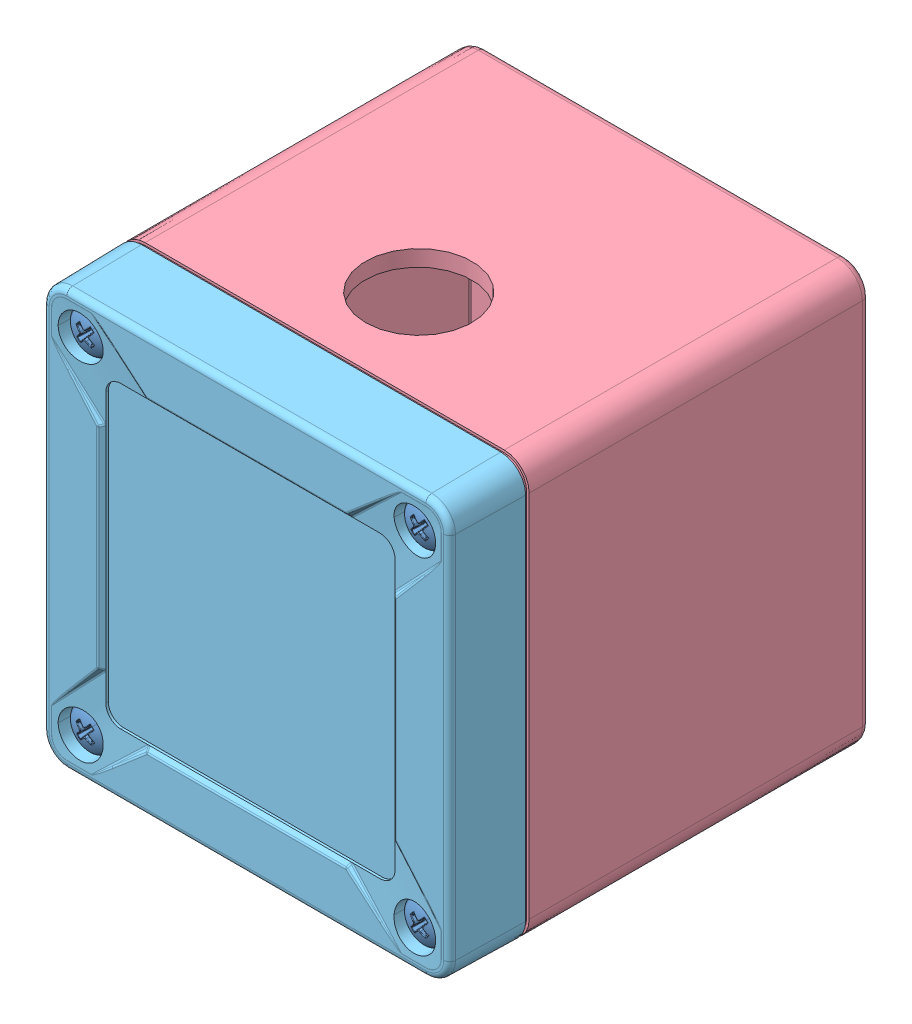
SolidWorks assembly SG-17, configuration Default. Lengths in mm.
Overall size (82 84 85.15).
14 component instances, 5 part files, 0 mates.
Components (placement in the parent):
- SG-17.STEP-1: SG-17.STEP [Default] at origin size (161.25 161.25 150.97)
  - SG-KIT-01.STEP-1: SG-KIT-01.STEP [Default] x (0.437882 0.496126 -0.749745) z (0.749745 -0.661726 0) size (120.85 121.81 107.11)
    - SCREWS-018_SCREWS-18.STEP-1: SCREWS-018_SCREWS-18.STEP [Default] at (-8.1241 12.1032 -47.946) x (0.749745 -0.661726 0) z (0 0 1) size (31.67 8.5 8.5)
    - SCREWS-018_SCREWS-18.STEP-2: SCREWS-018_SCREWS-18.STEP [Default] at (21.214 45.3437 2.2869) x (0.749745 -0.661726 0) z (0 0 1) size (31.67 8.5 8.5)
    - SCREWS-018_SCREWS-18.STEP-3: SCREWS-018_SCREWS-18.STEP [Default] at (-13.0187 6.5575 47.946) x (0.749745 -0.661726 0) z (0 0 1) size (31.67 8.5 8.5)
    - SCREWS-018_SCREWS-18.STEP-4: SCREWS-018_SCREWS-18.STEP [Default] at (-42.3568 -26.683 -2.2869) x (0.749745 -0.661726 0) z (0 0 1) size (31.67 8.5 8.5)
    - SCREWS-022_SCREWS-022.STEP-1: SCREWS-022_SCREWS-022.STEP [Default] at (43.0032 -34.1093 36.1352) x (0.749745 -0.661726 0) z (0 0 1) size (11.8 7.2 7.2)
    - SCREWS-022_SCREWS-022.STEP-2: SCREWS-022_SCREWS-022.STEP [Default] at (17.6061 -62.8846 -7.3501) x (0.749745 -0.661726 0) z (0 0 1) size (11.8 7.2 7.2)
    - SCREWS-022_SCREWS-022.STEP-3: SCREWS-022_SCREWS-022.STEP [Default] at (39.1876 -38.4325 -36.1352) x (0.749745 -0.661726 0) z (0 0 1) size (11.8 7.2 7.2)
    - SCREWS-022_SCREWS-022.STEP-4: SCREWS-022_SCREWS-022.STEP [Default] at (64.5847 -9.6571 7.3501) x (0.749745 -0.661726 0) z (0 0 1) size (11.8 7.2 7.2)
    - SG-98S.STEP-1: SG-98S.STEP [Default] at (27.4944 45.0649 2.533) x (0.041185 0.046663 -0.998061) z (0.660444 0.748292 0.062239) size (7.21 42.21 3.36)
    - SG-98S.STEP-2: SG-98S.STEP [Default] at (-4.2926 9.0498 -51.8929) x (-0.660444 -0.748292 -0.062239) z (0.041185 0.046663 -0.998061) size (7.21 42.21 3.36)
  - SG-17B_SG-17B-02.STEP-1: SG-17B_SG-17B-02.STEP [Default] at (0 0 1) size (82 84 71)
  - SG-10C_SG-10C-02.STEP-1: SG-10C_SG-10C-02.STEP [Default] at origin size (82 84 22.76)
